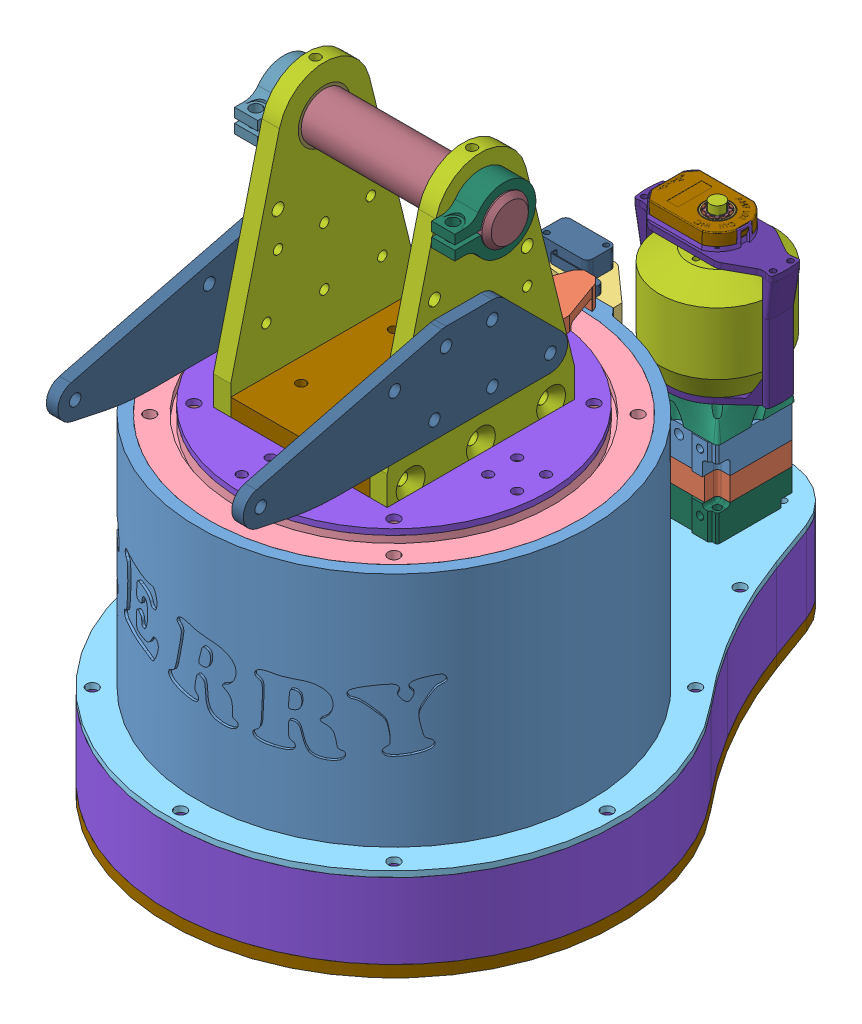
SolidWorks assembly Base, configuration Default. Lengths in mm.
Overall size (246.45 328.45 351.82).
86 component instances, 58 part files, 25 mates.
Components (placement in the parent):
- BotTurretHousing^Base-1: BotTurretHousing^Base [Default] at origin size (214.7 129.6 217.88) (virtual)
- SwitchTripper^Base-2: SwitchTripper^Base [Default] at origin size (28.57 11.52 54.14) (virtual)
- J1SwitchMount^Base-1: J1SwitchMount^Base [Default] at origin size (48.43 36.2 22.29) (virtual)
- 8in-1: 8in [Default] at (0 58.8 0) size (202 16 202)
- 8in-2: 8in [Default] at (0 -58.8 0) x (1 0 0) z (0 0 -1) size (202 16 202)
- BasePlate^Base-1: BasePlate^Base [Default] at origin size (246.45 3.17 338.52) (virtual)
- BotTurretPlate^Base-1: BotTurretPlate^Base [Default] at origin size (168.46 3.17 168.46) (virtual)
- SideTurretPlate^Base-1: SideTurretPlate^Base [Default] at origin size (9.52 279.65 102.6) (virtual)
- SideTurretPlate^Base-3: SideTurretPlate^Base [Default] x (-1 0 0) z (0 0 -1) size (9.52 279.65 102.6) (virtual)
- TopTurretPlate^Base-1: TopTurretPlate^Base [Default] at origin size (168.46 3.17 168.46) (virtual)
- TopBrace-1: TopBrace [Default] at origin size (76.2 9.53 102.6)
- PivotPlate^Base-1: PivotPlate^Base [Default] at origin size (6.35 50.8 177.8) (virtual)
- PivotPlate^Base-2: PivotPlate^Base [Default] at (101.6 0 0) size (6.35 50.8 177.8) (virtual)
- Keda9to1-1: Keda9to1 [Default] at (0 -48.175 -154.975) x (0 -1 0) z (1 0 0) size (176.96 63 76.93)
  - VersaPlanetary_v2_Single_Stage_10_1_with_BAG.STEP-1: VersaPlanetary_v2_Single_Stage_10_1_with_BAG.STEP [Default] at origin size (163.4 63.52 63.52)
    - 217-2820 Rev1_Public.STEP-1: 217-2820 Rev1_Public.STEP [Default] at (-4.6546 22.225 0) x (0 -0.456494 0.889726) z (-1 0 0) size (39.22 38.88 17.4)
      - 217-2625-100.STEP-1: 217-2625-100.STEP [Default] at origin size (39.22 38.88 12.7)
        - 217-2625-008 Rev1.STEP-1: 217-2625-008 Rev1.STEP [Default] at origin size (34.7 34.7 4.7)
        - 217-2625-010 Rev1.STEP-1: 217-2625-010 Rev1.STEP [Default] at (0 10.193 3.65) x (0.999813 0.019336 0) z (0 0 1) size (4 4 12)
        - 217-2625-010 Rev1.STEP-2: 217-2625-010 Rev1.STEP [Default] at (8.691 -5.3258 3.65) size (4 4 12)
        - 217-2625-010 Rev1.STEP-3: 217-2625-010 Rev1.STEP [Default] at (-8.691 -5.3258 3.65) size (4 4 12)
        - 217-2625-005 Rev1_Planet_Revolving_Follower01.STEP-1: 217-2625-005 Rev1_Planet_Revolving_Follower01.STEP [Default] at (8.691 -5.3258 6.35) x (0.932816 0.360354 0) z (0 0 1) size (16.89 16.89 8)
        - 217-2625-005 Rev1_Planet_Revolving_Follower01.STEP-2: 217-2625-005 Rev1_Planet_Revolving_Follower01.STEP [Default] at (-8.691 -5.3258 6.35) x (-0.932788 -0.360426 0) z (0 0 1) size (16.89 16.89 8)
        - 217-2625-005 Rev1_Planet_Revolving_Follower01.STEP-3: 217-2625-005 Rev1_Planet_Revolving_Follower01.STEP [Default] at (0 10.193 6.35) x (0.893583 0.448898 0) z (0 0 1) size (16.89 16.89 8)
      - 217-2625-007 Rev1_Public.STEP-1: 217-2625-007 Rev1_Public.STEP [Default] at (0 0 6.7) x (0.992772 0.120019 0) z (0 0 1) size (15.27 15.27 12.7)
    - 217-2625-026 Rev1.STEP-1: 217-2625-026 Rev1.STEP [Default] at (-6.5 22.225 0) x (0 -1 0) z (-1 0 0) size (44.45 42 18.12)
    - 217-2742-001 Rev4.STEP-1: 217-2742-001 Rev4.STEP [Default] at (0.2002 22.225 0) x (1 0 0) z (0 -0.092627 0.995701) size (7 28 28)
    - 217-2742-001 Rev4.STEP-2: 217-2742-001 Rev4.STEP [Default] at (8.2002 22.225 0) size (7 28 28)
    - 217-2625-017 Rev1_9714K61.STEP-1: 217-2625-017 Rev1_9714K61.STEP [Default] at (7.42 22.3002 -0.342) x (0 0.56703 0.823697) z (0 -0.823697 0.56703) size (28.51 4.98 27.43)
    - 217-2625-003 Rev1.STEP-1: 217-2625-003 Rev1.STEP [Default] at (7.4478 22.225 0) x (0 -1 0) z (1 0 0) size (17 17 64.11) (hidden)
    - 217-2625-018 Rev1_98541A410.STEP-1: 217-2625-018 Rev1_98541A410.STEP [Default] at (-0.7046 22.225 0) x (1 0 0) z (0 -0.017452 0.999848) size (1 19.6 17.4)
    - 832-1750-Ring-Gear-Screw_SSA0832-0500ZC.STEP-1: 832-1750-Ring-Gear-Screw_SSA0832-0500ZC.STEP [Default] at (-30.7 4.725 -17.5) x (0 0.997447 0.071411) z (0 -0.071411 0.997447) size (6.73 48.51 6.73) (hidden)
    - 832-1750-Ring-Gear-Screw_SSA0832-0500ZC.STEP-2: 832-1750-Ring-Gear-Screw_SSA0832-0500ZC.STEP [Default] at (-30.7 39.725 17.5) x (0 0.005929 0.999982) z (0 -0.999982 0.005929) size (6.73 48.51 6.73) (hidden)
    - 217-2625-025 Rev1.STEP-1: 217-2625-025 Rev1.STEP [Default] at (-23.2 22.225 0) x (0 -1 0) z (-1 0 0) size (44.45 42 18)
    - 217-4649-002 Rev1_SSA0832-0500ZC.STEP-1: 217-4649-002 Rev1_SSA0832-0500ZC.STEP [Default] at (-33.7 4.2645 17.9605) x (0 0.33842 -0.940995) z (0 0.940995 0.33842) size (6.73 16.76 6.73) (hidden)
    - 217-4649-002 Rev1_SSA0832-0500ZC.STEP-2: 217-4649-002 Rev1_SSA0832-0500ZC.STEP [Default] at (-33.7 40.1855 -17.9605) x (0 -0.308932 -0.951084) z (0 0.951084 -0.308932) size (6.73 16.76 6.73) (hidden)
    - 217-4649-006 Rev1_SSA0004-008BA.STEP-1: 217-4649-006 Rev1_SSA0004-008BA.STEP [Default] at (-30.7 22.225 12.5) x (0 0.5 -0.866025) z (0 -0.866025 -0.5) size (7 14 7) (hidden)
    - 217-4649-006 Rev1_SSA0004-008BA.STEP-2: 217-4649-006 Rev1_SSA0004-008BA.STEP [Default] at (-30.7 22.225 -12.5) x (0 -0.5 0.866025) z (0 0.866025 0.5) size (7 14 7) (hidden)
    - 217-2822-003 Rev4.STEP-1: 217-2822-003 Rev4.STEP [Default] at (-32.2 22.225 0) x (0 -1 0) z (-1 0 0) size (42 42 4.8) (hidden)
    - 217-3351 Rev2.STEP-1: 217-3351 Rev2.STEP [Default] at (-33.7 22.225 0) x (0 0 1) z (1 0 0) size (59.07 59.07 84.5) (hidden)
    - 217-2816-001 Rev1.STEP-1: 217-2816-001 Rev1.STEP [Default] at (-6.35 22.225 0) x (0 -1 0) z (1 0 0) size (42 42 14.51)
    - 217-4649-001 Rev1.STEP-1: 217-4649-001 Rev1.STEP [Default] at (-20.046 22.225 0) x (0 -1 0) z (1 0 0) size (18 18 13)
    - 217-4649-007 Rev1_94105A824.STEP-1: 217-4649-007 Rev1_94105A824.STEP [Default] at (-25.521 22.225 -6.7835) x (-0.996104 -0.088191 0) z (0 0 -1) size (4.83 4.83 4.77)
    - 217-2625-011 Rev1.STEP-1: 217-2625-011 Rev1.STEP [Default] at (-24.7818 22.225 0) x (0 0 1) z (0 -1 0) size (8.01 7.5 7.94) (hidden)
  - VersaPlanetary_CIM_Motor_Output_Shaft_Kit_217-2893-1: VersaPlanetary_CIM_Motor_Output_Shaft_Kit_217-2893 [Default] at (7.4478 22.225 0) x (0 0 -1) z (1 0 0) size (17 17 57.85)
  - KedaAdapter^Keda9to1-1: KedaAdapter^Keda9to1 [Default] at origin size (17.82 53.01 53.01) (virtual)
  - 192kvMotorEncoded-1: 192kvMotorEncoded [Default] at (-51.0318 22.225 0) x (0 -1 0) z (0 0 -1) size (63 104.52 76.93)
    - BetterKEDA-1: BetterKEDA [Default] at origin size (63 104.52 63)
    - CUI_DEVICES_AMT102-0048-N2000-S-1: CUI_DEVICES_AMT102-0048-N2000-S [Default] at (0 65.12 0) x (1 0 0) z (0 1 0) size (36.33 46.21 9.2)
      - CUI_DEVICES_AMT102-0048-N2000-S.step-1: CUI_DEVICES_AMT102-0048-N2000-S.step [Default] at origin size (36.33 46.21 9.2)
        - AMT-102-Base-REV-K.step-1: AMT-102-Base-REV-K.step [Default] x (-1 0 0) z (0 0 -1) size (28.78 43.39 9.06)
        - AMT-102-Top-Cover-REV-H.step-1: AMT-102-Top-Cover-REV-H.step [Default] at (0 0 5.23) x (-1 0 0) z (0 0 -1) size (28.6 43.26 6.55)
        - AMT-Sleeve-REV-D_ 2 mm.step-1: AMT-Sleeve-REV-D_ 2 mm.step [Default] at (0 0 -2.42) x (0.999996 0.002864 0) z (0 0 1) size (10.79 10.79 7.8)
        - AMT-Hub-Top-REV-D1.step-1: AMT-Hub-Top-REV-D1.step [Default] at (0 0 2.13) x (0.999996 0.002864 0) z (0 0 1) size (14 14 5.67)
        - AMT-Hub-Bottom-REV-B.step-1: AMT-Hub-Bottom-REV-B.step [Default] at (0 0 2.43) x (0.999998 -0.001942 0) z (0 0 1) size (17.3 17.3 3.2)
        - AMT10X-Shaft-Adaptor-REV-E.step-1: AMT10X-Shaft-Adaptor-REV-E.step [Default] at (0 0 0.03) x (0.999996 0.002864 0) z (0 0 1) size (11.8 11.8 7.8)
        - Receiver-board.step-1: Receiver-board.step [Default] at (72.2834 -20.351 3.03) x (-1 0 0) z (0 0 -1) size (26.5 26.62 0.41)
        - Rotor-board-REV F.step-1: Rotor-board-REV F.step [Default] at (0 0 2.13) x (0.807874 -0.589355 0) z (0 0 1) size (26 26 0.3)
        - Transmitter-board AMT10_AMT-102.step-1: Transmitter-board AMT10_AMT-102.step [Default] at (19.1596 -17.1102 1.22) x (-1 0 0) z (0 0 -1) size (26.63 38.43 4.41)
    - Body^192kvMotorEncoded-1: Body^192kvMotorEncoded [Default] at origin size (53 64.53 76.93) (virtual)
- J1Pulley-1: J1Pulley [Default] at (0 -94.5 0) size (144.9 24.53 144.9)
- 15Tpulley-2: 15Tpulley [Default] at (0 -86.5 -177.2) size (28 28 28)
- J1Belt133T^Base-1: J1Belt133T^Base [Default] at origin size (148.25 15.01 264.1) (virtual)
- TensionPillarJ1-1: TensionPillarJ1 [Default] at (5.0959 -4.9525 -9.5995) size (22.22 25.73 22.23)
  - 98019A228_MIL SPEC. 300 SERIES SS FLAT WASHER-1: 98019A228_MIL SPEC. 300 SERIES SS FLAT WASHER [98019A228] at (20.3041 -73.2587 -110.4505) x (0.972939 0 -0.231063) z (0.231063 0 0.972939) size (9.53 0.71 9.53)
  - 60355K701_BALL BEARING-1: 60355K701_BALL BEARING [60355K701] at (20.3041 -75.7479 -110.4505) x (1 0 0) z (0 1 0) size (15.88 15.88 4.98)
  - Roller^TensionPillarJ1-1: Roller^TensionPillarJ1 [Default] at (-2.0675 -15.5777 2.6827) size (22.23 15 22.23) (virtual)
  - 60355K701_BALL BEARING-2: 60355K701_BALL BEARING [60355K701] at (20.3041 -86.2673 -110.4505) x (1 0 0) z (0 1 0) size (15.88 15.88 4.98)
  - 375spacer-1: 375spacer [92510A777] at (20.3041 -67.785 -110.4505) x (1 0 0) z (0 -1 0) size (15.88 15.88 9.53)
- TensionPillarJ1-2: TensionPillarJ1 [Default] at (-5.0959 -4.9525 -230.5005) x (-1 0 0) z (0 0 -1) size (22.22 25.73 22.23)
  - 98019A228_MIL SPEC. 300 SERIES SS FLAT WASHER-1: 98019A228_MIL SPEC. 300 SERIES SS FLAT WASHER [98019A228] at (20.3041 -73.2587 -110.4505) x (0.972939 0 -0.231063) z (0.231063 0 0.972939) size (9.53 0.71 9.53)
  - 60355K701_BALL BEARING-1: 60355K701_BALL BEARING [60355K701] at (20.3041 -75.7479 -110.4505) x (1 0 0) z (0 1 0) size (15.88 15.88 4.98)
  - Roller^TensionPillarJ1-1: Roller^TensionPillarJ1 [Default] at (-2.0675 -15.5777 2.6827) size (22.23 15 22.23) (virtual)
  - 60355K701_BALL BEARING-2: 60355K701_BALL BEARING [60355K701] at (20.3041 -86.2673 -110.4505) x (1 0 0) z (0 1 0) size (15.88 15.88 4.98)
  - 375spacer-1: 375spacer [92510A777] at (20.3041 -67.785 -110.4505) x (1 0 0) z (0 -1 0) size (15.88 15.88 9.53)
- TensionConnector^Base-1: TensionConnector^Base [Default] at origin size (66.67 5.72 15.88) (virtual)
- Foot^Base-1: Foot^Base [Default] at origin size (246.45 41.28 338.52) (virtual)
- Sole^Base-1: Sole^Base [Default] at origin size (246.45 6.35 338.52) (virtual)
- switch-1: switch [Default] at (-34 69.95 -117.75) x (-1 0 0) z (0 0 -1) size (39.3 10.3 27.5)
- 94459A340_BRASS HEAT-SET INSERT FOR PLASTIC-1: 94459A340_BRASS HEAT-SET INSERT FOR PLASTIC [94459A340] at (0 52.1 -104.175) x (0.708984 0.705225 0) z (-0.705225 0.708984 0) size (7.22 6.55 7.22)
- 94459A340_BRASS HEAT-SET INSERT FOR PLASTIC-2: 94459A340_BRASS HEAT-SET INSERT FOR PLASTIC [94459A340] at (0 39.4 -104.175) x (0.708984 0.705225 0) z (-0.705225 0.708984 0) size (7.22 6.55 7.22)
- 6391K422_OIL-EMBEDDED SLEEVE BEARING-1: 6391K422_OIL-EMBEDDED SLEEVE BEARING [6391K422] at (-44.45 187.45 0) x (0 0 -1) z (1 0 0) size (28.63 28.63 12.7)
- 6061K603_HARDENED PRECISION STEEL SHAFT-1: 6061K603_HARDENED PRECISION STEEL SHAFT [6061K603] at (0 187.45 0) size (127 25.4 25.4)
- 6391K422_OIL-EMBEDDED SLEEVE BEARING-2: 6391K422_OIL-EMBEDDED SLEEVE BEARING [6391K422] at (44.45 187.45 0) x (0 0 -1) z (1 0 0) size (28.63 28.63 12.7)
- SideClamp-1: SideClamp [Default] at origin size (12.7 34.92 44.45)
- MirrorSideClamp-3: MirrorSideClamp [Default] x (-1 0 0) z (0 0 -1) size (12.7 34.92 44.45)
Mates (geometry in assembly coordinates):
- Concentric1: concentric aligned: cylinder of BotTurretHousing^Base-1 through (0 50.8 0) axis (0 -1 0) radius 86.77; cylinder of 8in-1 through (0 64.8 0) axis (0 -1 0) radius 70
- Coincident1: coincident anti-aligned: plane of BotTurretHousing^Base-1 through (0 50.8 0) normal (0 1 0); plane of 8in-1 through (0 50.8 0) normal (0 -1 0)
- Concentric4: concentric anti-aligned: cylinder of BasePlate^Base-1 through (0 -67.975 -177.2) axis (0 1 0) radius 10; cylinder of Keda9to1-1/VersaPlanetary_CIM_Motor_Output_Shaft_Kit_217-2893-1 through (0 -63.3752 -177.2) axis (0 -1 0) radius 8.5
- Concentric5: concentric aligned: cylinder of BasePlate^Base-1 through (17.9605 -67.975 -159.2395) axis (0 1 0) radius 1.9844; cylinder of Keda9to1-1/VersaPlanetary_v2_Single_Stage_10_1_with_BAG.STEP-1/217-2625-026 Rev1.STEP-1 through (17.9605 -48.175 -159.2395) axis (0 1 0) radius 2.0193
- Coincident2: coincident anti-aligned: plane of BasePlate^Base-1 through (0 -64.8 0) normal (0 1 0); plane of Keda9to1-1/VersaPlanetary_v2_Single_Stage_10_1_with_BAG.STEP-1/217-2625-026 Rev1.STEP-1 through (22.225 -64.8 -199.425) normal (0 -1 0)
- Coincident3: coincident aligned: plane of J1Pulley-1 through (0 -94.5 0) normal (0 0 1)
- Coincident4: coincident aligned: plane of J1Pulley-1 through (0 -94.5 0) normal (1 0 0)
- Coincident7: coincident anti-aligned: plane of BotTurretPlate^Base-1 through (0 -69.975 0) normal (0 -1 0); plane of J1Pulley-1 through (0 -69.975 0) normal (0 1 0)
- Concentric6: concentric anti-aligned: cylinder of Keda9to1-1/VersaPlanetary_CIM_Motor_Output_Shaft_Kit_217-2893-1 through (0 -141.9432 -177.2) axis (0 1 0) radius 3.975; cylinder of 15Tpulley-2 through (0 -78.5 -177.2) axis (0 -1 0) radius 4
- Coincident8: coincident anti-aligned: plane of J1Pulley-1 through (0 -94.5 0) normal (0 -1 0); plane of 15Tpulley-2 through (0 -94.5 -177.2) normal (0 1 0)
- Concentric13: concentric anti-aligned: cylinder of BotTurretHousing^Base-1 through (0 52.1 107.3573) axis (0 0 -1) radius 3.2639; cylinder of 94459A340_BRASS HEAT-SET INSERT FOR PLASTIC-1 through (0 52.1 -104.175) axis (0 0 1) radius 3.1623
- Coincident15: coincident aligned: plane of BotTurretHousing^Base-1 through (0 39.4 -110.525) normal (0 0 -1); plane of 94459A340_BRASS HEAT-SET INSERT FOR PLASTIC-1 through (2.5211 54.6078 -110.525) normal (0 0 -1)
- Concentric14: concentric anti-aligned: cylinder of BotTurretHousing^Base-1 through (0 39.4 107.3573) axis (0 0 -1) radius 3.2639; cylinder of 94459A340_BRASS HEAT-SET INSERT FOR PLASTIC-2 through (0 39.4 -104.175) axis (0 0 1) radius 3.1623
- Coincident16: coincident aligned: plane of BotTurretHousing^Base-1 through (0 39.4 -110.525) normal (0 0 -1); plane of 94459A340_BRASS HEAT-SET INSERT FOR PLASTIC-2 through (2.5211 41.9078 -110.525) normal (0 0 -1)
- Parallel1: parallel anti-aligned: plane of BotTurretHousing^Base-1 through (0 64.8 0) normal (0 1 0); plane of switch-1 through (-34 64.8 -117.75) normal (0 -1 0)
- Coincident19: coincident: line of switch-1 through (0 72.45 -109.85) axis (0 -1 0)
- Parallel2: parallel aligned: plane of switch-1 through (-34 75.1 -114.95) normal (0 0 1)
- Tangent1: tangent anti-aligned: cylinder of BotTurretHousing^Base-1 through (0 368.4317 0) axis (0 -1 0) radius 107.35; cylinder of switch-1 through (0 72.45 -109.85) axis (0 -1 0) radius 2.5
- Coincident22: coincident anti-aligned: plane of BotTurretHousing^Base-1 through (0 64.8 0) normal (0 1 0); plane of switch-1 through (-34 64.8 -117.75) normal (0 -1 0)
- Coincident23: coincident aligned: plane of SideTurretPlate^Base-1 through (-38.1 187.45 0) normal (1 0 0); plane of 6391K422_OIL-EMBEDDED SLEEVE BEARING-1 through (-38.1 187.45 0) normal (1 0 0)
- Concentric16: concentric aligned: cylinder of SideTurretPlate^Base-1 through (-38.1 187.45 0) axis (-1 0 0) radius 14.3129; cylinder of 6391K422_OIL-EMBEDDED SLEEVE BEARING-1 through (-38.1 187.45 0) axis (-1 0 0) radius 12.7
- Concentric17: concentric anti-aligned: cylinder of 6391K422_OIL-EMBEDDED SLEEVE BEARING-1 through (-38.1 187.45 0) axis (-1 0 0) radius 12.7; cylinder of 6061K603_HARDENED PRECISION STEEL SHAFT-1 through (-63.5 187.45 0) axis (1 0 0) radius 12.7
- Width1: width anti-aligned: plane of 6061K603_HARDENED PRECISION STEEL SHAFT-1 through (63.5 187.45 0) normal (1 0 0); plane of SideTurretPlate^Base-1 through (-63.5 187.45 0) normal (-1 0 0); plane of 6061K603_HARDENED PRECISION STEEL SHAFT-1 through (-47.625 187.45 0) normal (-1 0 0); plane of SideTurretPlate^Base-3 through (47.625 187.45 0) normal (1 0 0)
- Coincident24: coincident anti-aligned: plane of BasePlate^Base-1 through (0 -67.975 0) normal (0 -1 0); plane of TensionPillarJ1-1/375spacer-1 through (25.4 -67.975 -120.05) normal (0 1 0)
- Concentric18: concentric aligned: circle of BasePlate^Base-1; cylinder of TensionPillarJ1-1/375spacer-1 through (25.4 -77.5 -120.05) axis (0 1 0) radius 7.9375
